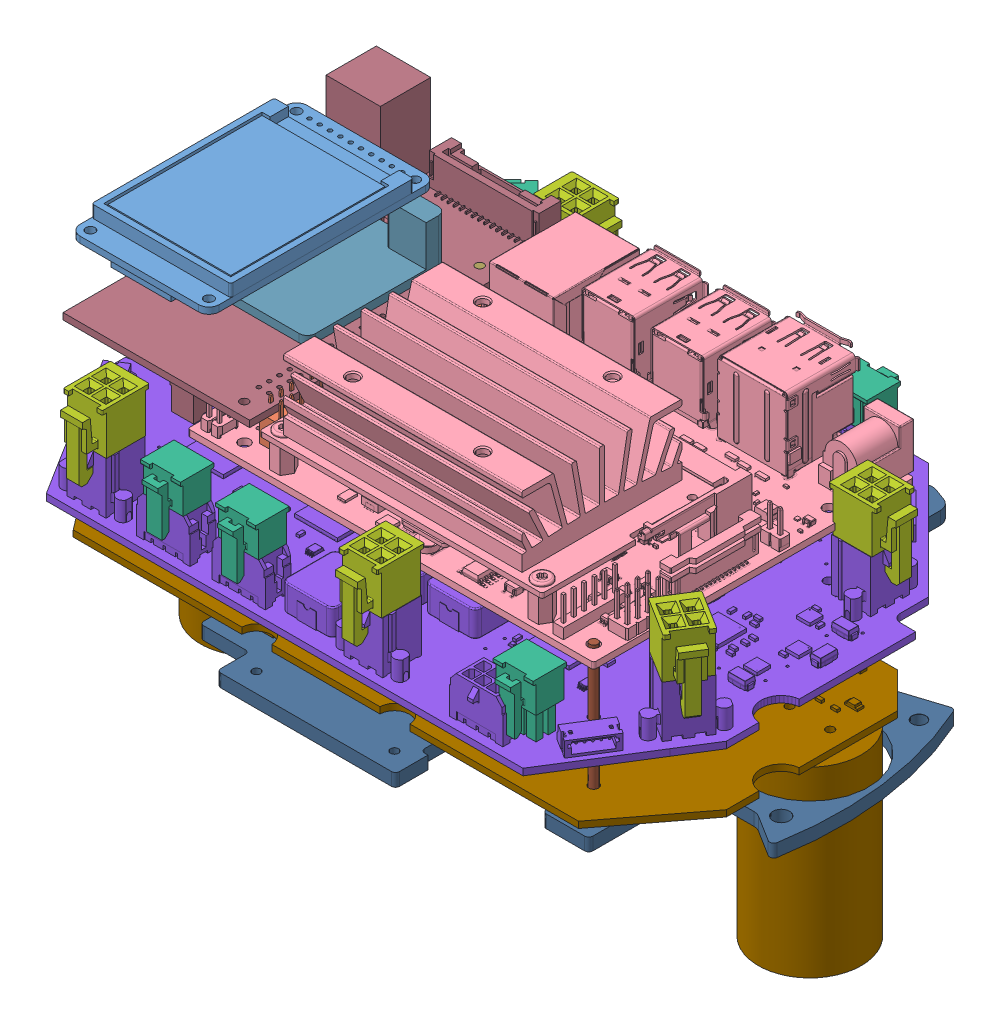
SolidWorks assembly ElecStack-v2.1, configuration Default. Lengths in mm.
Overall size (170.08 105.58 134.76).
26 component instances, 15 part files, 61 mates.
Components (placement in the parent):
- Adafruit 1.8 inch TFT Display-1: Adafruit 1.8 inch TFT Display [Default] at (-78.2449 69.1828 -26.0396) x (0 0 1) z (-1 0 0) size (55.88 6.57 34.29)
- PPTC202LFBN-RC--3DModel-STEP-1.step-1: PPTC202LFBN-RC--3DModel-STEP-1.step [Default] at (-29.0809 55.5828 4.0156) x (0 0 -1) z (-1 0 0) size (51.31 11.71 5.08)
- RockerSwitch-1: RockerSwitch [MR2-110-C5-BB3N] at (-63.8534 7.4427 -42.1881) x (0 1 0) z (-0.707107 0 -0.707107) size (24.12 21 37.37)
- Jetson nano 4GB-1: Jetson nano 4GB [Default] at (52.2561 46.8849 -26.7276) x (-1 0 0.000616) z (0 1 0) size (100 81.03 30.51)
- 430251008-2: 430251008 [Default] at (-73.6172 46.4899 -12.6558) x (-0.000616 0 -1) z (-1 0 0.000616) size (15.85 14 10.85)
- 430250600-1: 430250600 [Default] at (31.1451 46.4899 -56.3782) x (-1 0 0.000616) z (0.000616 0 1) size (9.85 14 10.85)
- 430250600-2: 430250600 [Default] at (-17.442 46.4899 45.623) x (1 0 -0.000616) z (-0.000616 0 -1) size (9.85 14 10.85)
- 430250600-3: 430250600 [Default] at (-51.9283 46.4899 -52.3019) x (-0.706671 0 0.707542) z (0.707542 0 0.706671) size (9.85 14 10.85)
- 430250600-4: 430250600 [Default] at (47.6097 44.1368 42.2998) x (1 0 -0.000616) z (-0.000616 0 -1) size (9.85 14 10.85)
- 430250600-5: 430250600 [Default] at (-35.984 46.4899 45.6345) x (1 0 -0.000616) z (-0.000616 0 -1) size (9.85 14 10.85)
- 39012040-1: 39012040 [Default] at (60.4916 45.6849 -29.068) x (-0.000616 0 -1) z (0 -1 0) size (9.6 14.4 19.6)
- 39012040-2: 39012040 [Default] at (64.596 45.6849 21.6996) x (0.530137 0 -0.847912) z (0 -1 0) size (9.6 14.4 19.6)
- 39012040-3: 39012040 [Default] at (-37.4917 45.6849 -54.1732) x (-0.000616 0 -1) z (0 -1 0) size (9.6 14.4 19.6)
- 39012040-5: 39012040 [Default] at (-54.8675 45.6849 44.2061) x (1 0 -0.000616) z (0 -1 0) size (9.6 14.4 19.6)
- 39012040-7: 39012040 [Default] at (13.1062 45.6849 44.3642) x (1 0 -0.000616) z (0 -1 0) size (9.6 14.4 19.6)
- motordriver-v5.1-18-03-22-1: motordriver-v5.1-18-03-22 [Default] at (54.555 32.8849 50.961) x (-0.000616 0 -1) z (0 1 0) size (115.09 156 16.89)
- power-v3.5-1: power-v3.5 [Default] at (-155.166 18.2579 93.3202) x (1 0 -0.000616) z (0 1 0) size (162.76 87.14 57.13)
- MidPlate_Alt2-1: MidPlate_Alt2 [Default] at (-4.1698 7.5266 -1.3119) x (1 0 -0.000616) z (0.000616 0 1) size (170 3.25 127.43)
- Standoff-mockup-for wireframe-1: Standoff-mockup-for wireframe [Default] at (56.686 10.7016 -25.4158) size (2 38.19 2)
- Standoff-mockup-for wireframe-3: Standoff-mockup-for wireframe [Default] at (52.2919 10.7016 31.2724) size (2 38.19 2)
- Standoff-mockup-for wireframe UI-1: Standoff-mockup-for wireframe UI [Default] at (-33.7439 6.3328 -26.6746) size (2 50.85 2)
- Standoff-mockup-for wireframe UI-2: Standoff-mockup-for wireframe UI [Default] at (-33.7081 6.3328 31.3254) size (2 50.85 2) (hidden)
- Standoff-mockup-for wireframe UI-3: Standoff-mockup-for wireframe UI [Default] at (-79.1876 10.7016 -30.2657) size (2 50.85 2)
- ui_layout-v1.0-1: ui_layout-v1.0 [Default] at (-28.0799 57.1828 34.6664) x (0 0 -1) z (0 1 0) size (78.99 54.1 29.21)
- ScreenSupport_PowerSwitch-1: ScreenSupport_PowerSwitch [Default] at (-37.4939 57.1828 -22.2296) x (-1 0 0) z (0 0 -1) size (30 12 34.29)
- DA102J12S217HQF-1: DA102J12S217HQF [Default] at (-83.1979 63.2153 26.4149) x (0 0 -1) z (0 1 0) size (21 20.6 15)
Mates (geometry in assembly coordinates):
- Parallel9: parallel aligned: plane of RockerSwitch-1 through (-47.9789 13.8927 -38.6879) normal (0 1 0)
- Concentric28: concentric anti-aligned: cylinder of MidPlate_Alt2-1 through (52.2561 7.5266 -26.7276) axis (0 -1 0) radius 1.2; cylinder of Jetson nano 4GB-1 through (52.2561 46.8849 -26.7276) axis (0 1 0) radius 1.375
- Concentric33: concentric anti-aligned: cylinder of Jetson nano 4GB-1 through (-33.7081 46.8849 31.3254) axis (0 1 0) radius 1.375; cylinder of MidPlate_Alt2-1 through (-33.7081 7.5266 31.3254) axis (0 -1 0) radius 1.2
- Concentric39: concentric anti-aligned: cylinder of MidPlate_Alt2-1 through (74.3767 7.5266 7.1413) axis (0 1 0) radius 2.05; cylinder of NETPS8_68_F8_G8_SC0_M4_N4-1 through (78.8065 -1.2244 8.4531) axis (0 -1 0) radius 2
- Coincident83: coincident anti-aligned: plane of MidPlate_Alt2-1 through (-4.1698 10.7016 -1.3119) normal (0 1 0); plane of NETPS8_68_F8_G8_SC0_M4_N4-1 through (82.3065 6.7756 8.4531) normal (0 -1 0)
- Coincident84: coincident anti-aligned: plane of MidPlate_Alt2-1 through (-4.1698 10.7016 -1.3119) normal (0 1 0); plane of NETPS8_68_F8_G8_SC0_M4_N4-2 through (-74.8386 6.7756 7.8903) normal (0 -1 0)
- Concentric40: concentric anti-aligned: cylinder of MidPlate_Alt2-1 through (-82.7057 7.5266 7.2381) axis (0 1 0) radius 2.05; cylinder of NETPS8_68_F8_G8_SC0_M4_N4-2 through (-78.2759 -1.2244 8.5499) axis (0 -1 0) radius 2
- Concentric45: concentric aligned: cylinder of MidPlate_Alt2-1 through (52.2919 7.5266 31.2724) axis (0 -1 0) radius 1.2; cylinder of Standoff-mockup-for wireframe-3 through (52.2919 48.8916 31.2724) axis (0 -1 0) radius 1
- Coincident89: coincident anti-aligned: plane of MidPlate_Alt2-1 through (-4.1698 10.7016 -1.3119) normal (0 1 0); plane of Standoff-mockup-for wireframe-3 through (52.2919 10.7016 31.2724) normal (0 -1 0)
- Coincident90: coincident anti-aligned: plane of MidPlate_Alt2-1 through (-4.1698 10.7016 -1.3119) normal (0 1 0); plane of Standoff-mockup-for wireframe-1 through (56.686 10.7016 -25.4158) normal (0 -1 0)
- Concentric51: concentric anti-aligned: cylinder of Standoff-mockup-for wireframe UI-2 through (-33.7081 57.1828 31.3254) axis (0 -1 0) radius 1; circle of Jetson nano 4GB-1
- Concentric56: concentric anti-aligned: cylinder of MidPlate_Alt2-1 through (-79.1876 10.7016 -30.2657) axis (0 1 0) radius 1.7; cylinder of Standoff-mockup-for wireframe UI-3 through (-79.1876 61.5516 -30.2657) axis (0 -1 0) radius 1
- Coincident93: coincident anti-aligned: plane of MidPlate_Alt2-1 through (-4.1698 10.7016 -1.3119) normal (0 1 0); plane of Standoff-mockup-for wireframe UI-3 through (-79.1876 10.7016 -30.2657) normal (0 -1 0)
- Concentric57: concentric aligned: cylinder of MidPlate_Alt2-1 through (52.2919 7.5266 31.2724) axis (0 -1 0) radius 1.2; cylinder of motordriver-v5.1-18-03-22-1 through (52.2919 31.2579 31.2724) axis (0 -1 0) radius 1.2
- Concentric58: concentric aligned: cylinder of MidPlate_Alt2-1 through (-33.7439 7.5266 -26.6746) axis (0 -1 0) radius 1.2; cylinder of motordriver-v5.1-18-03-22-1 through (-33.7439 31.2579 -26.6746) axis (0 -1 0) radius 1.2
- Distance11: distance = 14 mm anti-aligned: plane of motordriver-v5.1-18-03-22-1 through (73.8391 32.8849 12.1121) normal (0 1 0); plane of Jetson nano 4GB-1 through (52.2561 46.8849 -26.7276) normal (0 -1 0)
- Coincident99: coincident anti-aligned: plane of 430251008-2 through (-76.3127 42.8399 -5.4541) normal (-1 0 0.000616); plane of motordriver-v5.1-18-03-22-1 through (-76.3142 42.8399 -7.8541) normal (1 0 -0.000616)
- Coincident100: coincident anti-aligned: plane of 430251008-2 through (-73.3216 42.8399 -19.856) normal (-0.000616 0 -1); plane of motordriver-v5.1-18-03-22-1 through (-70.7816 42.8399 -19.8575) normal (0.000616 0 1)
- Coincident101: coincident anti-aligned: plane of 430251008-2 through (-70.192 42.8399 -20.5779) normal (0 -1 0); plane of motordriver-v5.1-18-03-22-1 through (-70.1229 42.8399 -21.9129) normal (0 1 0)
- Coincident102: coincident anti-aligned: plane of 430250600-5 through (-31.7839 42.8399 45.9319) normal (1 0 -0.000616); plane of motordriver-v5.1-18-03-22-1 through (-31.7824 42.8399 48.3319) normal (-1 0 0.000616)
- Coincident103: coincident anti-aligned: plane of 430250600-5 through (-37.7824 42.8399 48.3356) normal (0.000616 0 1); plane of motordriver-v5.1-18-03-22-1 through (-40.3224 42.8399 48.3371) normal (-0.000616 0 -1)
- Coincident104: coincident anti-aligned: plane of 430250600-5 through (-31.0619 42.8399 49.0614) normal (0 -1 0); plane of motordriver-v5.1-18-03-22-1 through (-29.727 42.8399 48.9906) normal (0 1 0)
- Coincident105: coincident anti-aligned: plane of 39012040-5 through (-51.0673 45.6849 44.5037) normal (1 0 -0.000616); plane of motordriver-v5.1-18-03-22-1 through (-51.0651 45.6849 48.1037) normal (-1 0 0.000616)
- Coincident106: coincident anti-aligned: plane of 39012040-5 through (-58.6699 45.6849 40.3084) normal (-0.000616 0 -1); plane of motordriver-v5.1-18-03-22-1 through (-55.2699 45.6849 40.3063) normal (0.000616 0 1)
- Coincident107: coincident anti-aligned: plane of 39012040-5 through (-59.6646 45.6849 49.009) normal (0 -1 0); plane of motordriver-v5.1-18-03-22-1 through (-50.1646 45.6849 49.0032) normal (0 1 0)
- Coincident108: coincident anti-aligned: plane of 430250600-2 through (-13.2419 42.8399 45.9204) normal (1 0 -0.000616); plane of motordriver-v5.1-18-03-22-1 through (-13.2404 42.8399 48.3204) normal (-1 0 0.000616)
- Coincident109: coincident anti-aligned: plane of 430250600-2 through (-19.2404 42.8399 48.3241) normal (0.000616 0 1); plane of motordriver-v5.1-18-03-22-1 through (-21.7804 42.8399 48.3257) normal (-0.000616 0 -1)
- Coincident110: coincident anti-aligned: plane of 430250600-2 through (-12.5199 42.8399 49.05) normal (0 -1 0); plane of motordriver-v5.1-18-03-22-1 through (-11.185 42.8399 48.9792) normal (0 1 0)
- Coincident111: coincident anti-aligned: plane of 39012040-7 through (16.9085 45.6849 48.0619) normal (0.000616 0 1); plane of motordriver-v5.1-18-03-22-1 through (13.5085 45.6849 48.064) normal (-0.000616 0 -1)
- Coincident112: coincident anti-aligned: plane of 39012040-7 through (9.3059 45.6849 43.8666) normal (-1 0 0.000616); plane of motordriver-v5.1-18-03-22-1 through (9.3037 45.6849 40.2666) normal (1 0 -0.000616)
- Coincident113: coincident anti-aligned: plane of 39012040-7 through (8.3091 45.6849 49.1672) normal (0 -1 0); plane of motordriver-v5.1-18-03-22-1 through (18.009 45.6849 48.9612) normal (0 1 0)
- Coincident114: coincident anti-aligned: plane of 430250600-3 through (-55.1086 42.8399 -49.5422) normal (-0.706671 0 0.707542); plane of motordriver-v5.1-18-03-22-1 through (-56.8067 42.8399 -51.2383) normal (0.706671 0 -0.707542)
- Coincident115: coincident anti-aligned: plane of 430250600-3 through (-52.5666 42.8399 -55.4835) normal (-0.707542 0 -0.706671); plane of motordriver-v5.1-18-03-22-1 through (-50.7717 42.8399 -57.2807) normal (0.707542 0 0.706671)
- Coincident116: coincident anti-aligned: plane of 39012040-3 through (-33.7894 45.6849 -50.3755) normal (0.000616 0 1); plane of motordriver-v5.1-18-03-22-1 through (-36.4894 45.6849 -50.3739) normal (-0.000616 0 -1)
- Coincident117: coincident anti-aligned: plane of 39012040-3 through (-33.7941 45.6849 -57.9755) normal (1 0 -0.000616); plane of motordriver-v5.1-18-03-22-1 through (-33.792 45.6849 -54.5755) normal (-1 0 0.000616)
- Coincident118: coincident anti-aligned: plane of 430250600-1 through (35.3452 42.8399 -56.0808) normal (1 0 -0.000616); plane of motordriver-v5.1-18-03-22-1 through (35.3468 42.8399 -53.5408) normal (-1 0 0.000616)
- Coincident119: coincident anti-aligned: plane of 430250600-1 through (26.9434 42.8399 -59.0756) normal (-0.000616 0 -1); plane of motordriver-v5.1-18-03-22-1 through (29.3434 42.8399 -59.0771) normal (0.000616 0 1)
- Coincident120: coincident anti-aligned: plane of 430250600-1 through (26.2229 42.8399 -59.8051) normal (0 -1 0); plane of motordriver-v5.1-18-03-22-1 through (24.748 42.8399 -59.7342) normal (0 1 0)
- Coincident121: coincident anti-aligned: plane of 39012040-3 through (-32.6888 45.6849 -49.3762) normal (0 -1 0); plane of motordriver-v5.1-18-03-22-1 through (-32.8947 45.6849 -59.0761) normal (0 1 0)
- Coincident122: coincident anti-aligned: plane of 430250600-3 through (-57.832 42.8399 -51.2447) normal (0 -1 0); plane of motordriver-v5.1-18-03-22-1 through (-58.7259 42.8399 -50.2507) normal (0 1 0)
- Coincident123: coincident anti-aligned: plane of 39012040-1 through (60.7892 45.6849 -32.8682) normal (-0.000616 0 -1); plane of motordriver-v5.1-18-03-22-1 through (64.1892 45.6849 -32.8703) normal (0.000616 0 1)
- Coincident124: coincident anti-aligned: plane of 39012040-1 through (64.1918 45.6849 -28.6703) normal (1 0 -0.000616); plane of motordriver-v5.1-18-03-22-1 through (64.194 45.6849 -25.0703) normal (-1 0 0.000616)
- Coincident125: coincident anti-aligned: plane of 39012040-1 through (65.2945 45.6849 -24.2709) normal (0 -1 0); plane of motordriver-v5.1-18-03-22-1 through (65.0887 45.6849 -33.7708) normal (0 1 0)
- Coincident126: coincident anti-aligned: plane of 39012040-2 through (67.5212 45.6849 24.0003) normal (0.847912 0 0.530137); plane of motordriver-v5.1-18-03-22-1 through (65.7188 45.6849 26.8832) normal (-0.847912 0 -0.530137)
- Coincident127: coincident anti-aligned: plane of 39012040-2 through (62.1575 45.6849 24.6566) normal (-0.530137 0 0.847912); plane of motordriver-v5.1-18-03-22-1 through (59.105 45.6849 22.7481) normal (0.530137 0 -0.847912)
- Coincident128: coincident anti-aligned: plane of 39012040-2 through (66.1213 45.6849 28.3143) normal (0 -1 0); plane of motordriver-v5.1-18-03-22-1 through (71.0941 45.6849 19.9835) normal (0 1 0)
- Concentric67: concentric anti-aligned: cylinder of Jetson nano 4GB-1 through (-33.7439 46.8849 -26.6746) axis (0 1 0) radius 1.375; cylinder of ui_layout-v1.0-1 through (-33.7439 55.5828 -26.6746) axis (0 -1 0) radius 1
- Parallel10: parallel anti-aligned: cylinder of Jetson nano 4GB-1 through (-33.7081 46.8849 31.3254) axis (0 1 0) radius 1.375; cylinder of ui_layout-v1.0-1 through (-33.7439 55.5828 31.3394) axis (0 -1 0) radius 1
- Coincident138: coincident anti-aligned: plane of PPTC202LFBN-RC--3DModel-STEP-1.step-1 through (-29.0809 55.5828 4.0156) normal (0 1 0); plane of ui_layout-v1.0-1 through (-83.1979 55.5828 1.5194) normal (0 -1 0)
- Concentric69: concentric aligned: cylinder of Adafruit 1.8 inch TFT Display-1 through (-72.5299 69.1828 -23.4996) axis (0 1 0) radius 0.5; circle of ui_layout-v1.0-1
- Concentric70: concentric aligned: cylinder of Adafruit 1.8 inch TFT Display-1 through (-49.6699 69.1828 -23.4996) axis (0 1 0) radius 0.5; circle of ui_layout-v1.0-1
- Concentric71: concentric anti-aligned: circle of MidPlate_Alt2-1; circle of power-v3.5-1
- Concentric73: concentric aligned: cylinder of power-v3.5-1 through (-33.7081 16.7016 31.3254) axis (0 -1 0) radius 1.2; cylinder of MidPlate_Alt2-1 through (-33.7081 7.5266 31.3254) axis (0 -1 0) radius 1.2
- Distance12: distance = 6 mm anti-aligned: plane of power-v3.5-1 through (-82.152 16.7016 20.2122) normal (0 -1 0); plane of MidPlate_Alt2-1 through (-4.1698 10.7016 -1.3119) normal (0 1 0)
- Distance14: distance = 13 mm anti-aligned: plane of motordriver-v5.1-18-03-22-1 through (73.8391 31.2579 12.1121) normal (0 -1 0); plane of power-v3.5-1 through (-82.152 18.2579 20.2122) normal (0 1 0)
- Concentric74: concentric aligned: cylinder of MidPlate_Alt2-1 through (-33.7439 7.5266 -26.6746) axis (0 -1 0) radius 1.2; cylinder of Standoff-mockup-for wireframe UI-1 through (-33.7439 57.1828 -26.6746) axis (0 -1 0) radius 1
- Coincident139: coincident anti-aligned: plane of ui_layout-v1.0-1 through (-83.1979 57.1828 1.5194) normal (0 1 0); plane of ScreenSupport_PowerSwitch-1 through (-37.4939 57.1828 -22.2296) normal (0 -1 0)
- Coincident141: coincident anti-aligned: plane of Adafruit 1.8 inch TFT Display-1 through (-78.2449 69.1828 -26.0396) normal (0 -1 0); plane of ScreenSupport_PowerSwitch-1 through (-37.4939 69.1828 -22.2296) normal (0 1 0)
- Coincident143: coincident anti-aligned: plane of ui_layout-v1.0-1 through (-83.1979 57.1828 1.5194) normal (0 1 0); plane of DA102J12S217HQF-1 through (-72.7519 57.1828 34.9239) normal (0 -1 0)
- Coincident148: coincident anti-aligned: plane of ui_layout-v1.0-1 through (-83.1979 55.5828 -27.3096) normal (-1 0 0); plane of DA102J12S217HQF-1 through (-83.1979 63.2153 26.4149) normal (1 0 0)
- Coincident149: coincident anti-aligned: plane of ui_layout-v1.0-1 through (-60.6239 57.1828 -22.2296) normal (0 0 1); plane of ScreenSupport_PowerSwitch-1 through (-37.4939 59.1828 -22.2296) normal (0 0 -1)
